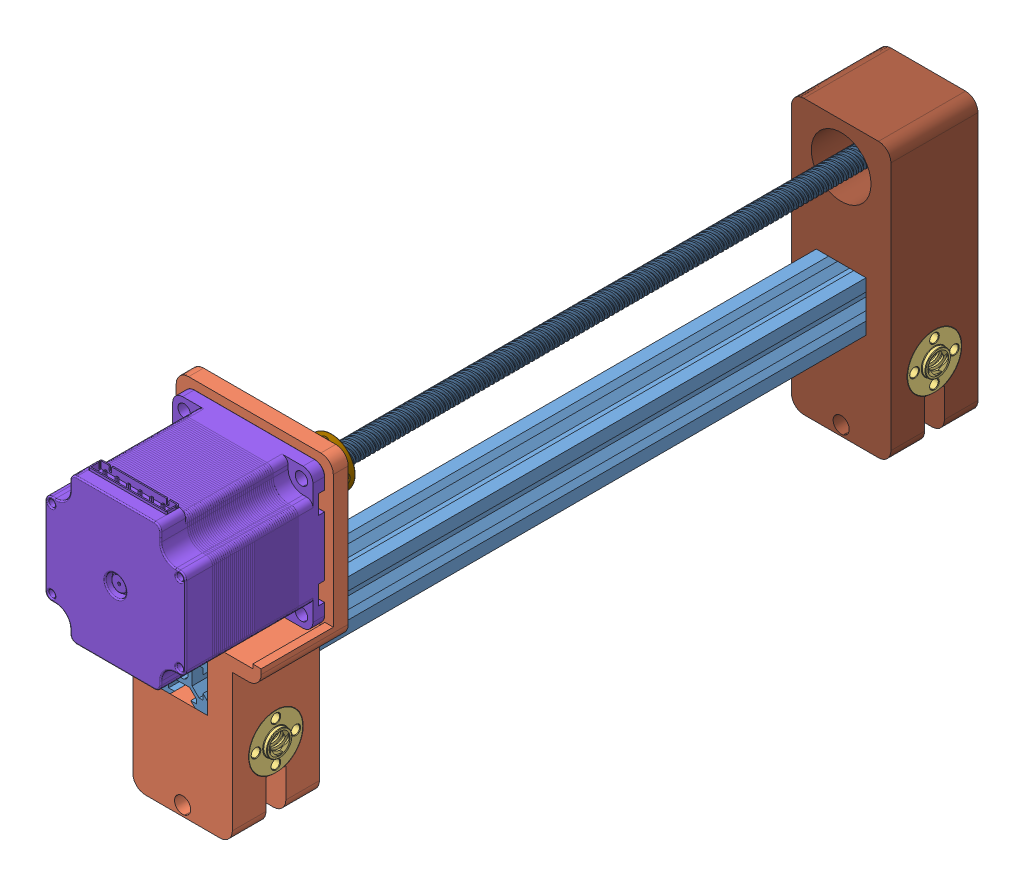
SolidWorks assembly AxisY, configuration Predeterminado. Lengths in mm.
Overall size (63.14 134.08 330.34).
24 component instances, 14 part files, 10 mates.
Components (placement in the parent):
- BoschAxisY-1: BoschAxisY [Predeterminado] at (-10.2409 9.7323 149.855) size (20 20 299.71)
- NEMA-SupportY-1: NEMA-SupportY [Predeterminado] at (-5.3102 -11.7496 522.235) x (-1 0 0) z (0 0 -1) size (63.14 134.08 76.6)
  - NEMA-SupportY-1: NEMA-SupportY [Predeterminado] at (-25.0692 -38.6881 72.67) size (63.14 125.31 35)
  - T8-Screw-1: T8-Screw [Default] at (-25.0692 -11.3281 90.17) x (0 0 -1) z (-1 0 0) size (22 22 16.4)
  - skf_bearing_61901_2-1: skf_bearing_61901_2 [Default] at (-5.0692 -34.6881 93.1623) x (0 0 -1) z (0.997819 -0.066004 0) size (6 24 24)
    - skf_bearing_61901_2_01-1: skf_bearing_61901_2_01 [Default] at origin size (6 24 24)
    - skf_bearing_61901_2_02-1: skf_bearing_61901_2_02 [Default] at origin size (6 16 16)
    - skf_bearing_61901_2_03-1: skf_bearing_61901_2_03 [Default] at origin size (3.18 21.18 20.29)
    - PiezaInterna-1: PiezaInterna [Predeterminado] x (0 0 -1) z (1 0 0) size (12 12 6)
  - Nema 23-1: Nema 23 [Default] at (-5.0692 55.0519 45.67) size (56.4 59.4 76.6)
- Coupler 6.35-8mm-1: Coupler 6.35-8mm [Default] at (-0.2409 43.3023 402.065) size (19.34 19.34 25)
- ScrewAxisY-1: ScrewAxisY [Default] at (-0.2409 43.3023 547.965) x (0.923728 0.383049 0) z (0 0 1) size (8.33 8.33 255.98)
- SupportY-2: SupportY [Predeterminado] at (-14.2503 2.2878 277.525) x (-1 0 0) z (0 0 -1) size (42.2 118.83 35)
  - SupportY-1: SupportY [Predeterminado] at (-34.0094 -52.7255 92.67) size (40 110.17 35)
  - skf_bearing_61901_2-1: skf_bearing_61901_2 [Default] at (-14.0094 -48.7255 113.1765) x (0 0 -1) z (0.998419 -0.056205 0) size (6 24 24)
    - skf_bearing_61901_2_01-1: skf_bearing_61901_2_01 [Default] at origin size (6 24 24)
    - skf_bearing_61901_2_02-1: skf_bearing_61901_2_02 [Default] at origin size (6 16 16)
    - skf_bearing_61901_2_03-1: skf_bearing_61901_2_03 [Default] at origin size (3.18 21.18 20.29)
    - PiezaInterna-1: PiezaInterna [Predeterminado] x (0 0 -1) z (1 0 0) size (12 12 6)
  - skf_bearing_609_2-1: skf_bearing_609_2 [Default] at (-14.0094 41.0145 117.67) x (0 0 -1) z (0 -1 0) size (7 24 24)
    - skf_bearing_609_2_01-1: skf_bearing_609_2_01 [Default] at origin size (7 24 24)
    - skf_bearing_609_2_02-1: skf_bearing_609_2_02 [Default] at origin size (7 14.45 14.45)
    - skf_bearing_609_2_03-1: skf_bearing_609_2_03 [Default] at origin size (3.97 20.97 20.97)
  - T8-Screw-1: T8-Screw [Default] at (-34.0094 -25.3655 110.17) x (0 1 0) z (-1 0 0) size (22 22 16.4)
Mates (geometry in assembly coordinates):
- Coincidente4: coincident anti-aligned: plane of BoschAxisY-1 through (-10.2409 -10.2677 449.565) normal (0 -1 0); plane of ScrewSupport&NEMA-1/ScrewSupportY2-1 through (19.7591 -10.2677 414.565) normal (0 1 0)
- Coincidente5: coincident aligned: plane of BoschAxisY-1 through (-10.2409 9.7323 449.565) normal (0 0 1); plane of ScrewSupport&NEMA-1/ScrewSupportY2-1 through (19.7591 -50.4377 449.565) normal (0 0 1)
- Coincidente6: coincident anti-aligned: plane of BoschAxisY-1 through (-10.2409 9.7323 449.565) normal (-1 0 0); plane of ScrewSupport&NEMA-1/ScrewSupportY2-1 through (-10.2409 -50.4377 414.565) normal (1 0 0)
- Concéntrica1: concentric anti-aligned: cylinder of NEMA-SupportY-1/Nema 23-1 through (-0.2409 43.3023 414.965) axis (0 0 1) radius 3.175; circle of Coupler 6.35-8mm-1
- Coincidente7: coincident anti-aligned: plane of NEMA-SupportY-1/NEMA-SupportY-1 through (19.7591 -50.4377 414.565) normal (0 0 -1); plane of Coupler 6.35-8mm-1 through (-0.2409 43.3023 414.565) normal (0 0 1)
- Coincidente8: coincident anti-aligned: plane of NEMA-SupportY-1/Nema 23-1 through (-0.2409 43.3023 399.965) normal (0 0 -1); plane of ScrewAxisY-1 through (-0.2409 43.3023 399.965) normal (0 0 1)
- Concéntrica2: concentric anti-aligned: circle of Coupler 6.35-8mm-1; circle of ScrewAxisY-1
- Coincidente9: coincident anti-aligned: plane of BoschAxisY-1 through (-10.2409 9.7323 449.565) normal (-1 0 0); plane of SupportY-2/SupportY-1 through (-10.2409 -50.4377 149.855) normal (1 0 0)
- Coincidente10: coincident aligned: plane of BoschAxisY-1 through (-10.2409 9.7323 149.855) normal (0 0 -1); plane of SupportY-2/SupportY-1 through (19.7591 -50.4377 149.855) normal (0 0 -1)
- Coincidente11: coincident anti-aligned: plane of BoschAxisY-1 through (-10.2409 9.7323 449.565) normal (0 1 0); plane of SupportY-2/SupportY-1 through (19.7591 9.7323 149.855) normal (0 -1 0)
